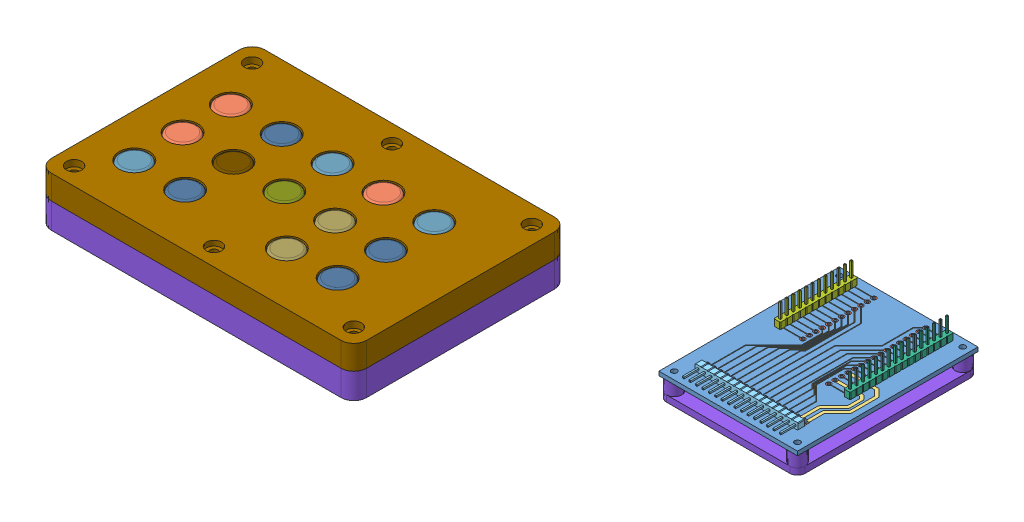
SolidWorks assembly central_station, configuration Default. Lengths in mm.
Overall size (285.1 66.66 84.42).
110 component instances, 27 part files, 11 mates.
Components (placement in the parent):
- controller1-controller.step-1: controller1-controller.step [Default] at (-1.9609 35.1675 90.037) x (1 0 0) z (0 1 0) size (54.5 71 11.54)
  - Board_Geoms_2cbe.step-1: Board_Geoms_2cbe.step [Default] at origin size (54.5 71 1.65)
    - Pcb_2cbe.step-1: Pcb_2cbe.step [Default] at (-119.5 126 0) size (54.5 71 1.6)
    - topPads_2cbe.step-1: topPads_2cbe.step [Default] at (-119.5 126 0.02) size (39.81 57.72 0.01)
    - topTracks_2cbe.step-1: topTracks_2cbe.step [Default] at (-119.5 126 0.01) size (44.1 56.73 0.01)
    - botPads_2cbe.step-1: botPads_2cbe.step [Default] at (-119.5 126 -1.62) size (39.81 57.72 0.01)
  - Step_Models_2cbe.step-1: Step_Models_2cbe.step [Default] at origin size (40.64 67.26 11.54)
    - Top_2cbe.step-1: Top_2cbe.step [Default] at origin size (40.64 67.26 11.54)
      - J3_PinHeader_1x16_P254mm_Horizontal_6185DDD9.step-1: J3_PinHeader_1x16_P254mm_Horizontal_6185DDD9.step [Default] at (46.34 11.21 0) x (0 -1 0) z (0 0 1) size (10.36 40.64 5.54)
      - J2_PinHeader_1x16_P254mm_Vertical_6185DCF0.step-1: J2_PinHeader_1x16_P254mm_Vertical_6185DCF0.step [Default] at (46.14 29.06 0) x (-1 0 0) z (0 0 1) size (2.54 40.64 11.54)
      - J1_PinHeader_1x12_P254mm_Vertical_6185DCCC.step-1: J1_PinHeader_1x12_P254mm_Vertical_6185DCCC.step [Default] at (8.52 67.16 0) size (2.54 30.48 11.54)
- base-1: base [Default] at (68.1365 26.0675 3.2619) size (54.5 7.5 71)
- Control_pad1-Control_pad.step-1: Control_pad1-Control_pad.step [Default] at (-325.562 -13.3521 -38.5409) x (1 0 0) z (0 1 0) size (120 80 13.4)
  - Board_Geoms_9430.step-1: Board_Geoms_9430.step [Default] at origin size (120 80 1.6)
    - Pcb_9430.step-1: Pcb_9430.step [Default] at origin size (120 80 1.6)
  - Step_Models_9430.step-1: Step_Models_9430.step [Default] at origin size (106.29 65.25 13.4)
    - Top_9430.step-1: Top_9430.step [Default] at origin size (106.29 65.25 13.4)
      - S2__2mmx12mm_With_White_cap_round_6188A434.step-1: S2__2mmx12mm_With_White_cap_round_6188A434.step [Default] at (130 -83.35 0) size (13.42 13 13.05)
        - round-cap.step-1: round-cap.step [Default] at origin size (13 13 7.7)
        - Tactal_Switch_-_THRU(12mmx12mmx__mm)-Square_Yellow.step-1: Tactal_Switch_-_THRU(12mmx12mmx__mm)-Square_Yellow.step [Default] at origin size (13.42 12.01 10.79)
      - S2__2mmx12mm_With_White_cap_round_6188A434.step-2: S2__2mmx12mm_With_White_cap_round_6188A434.step [Default] at (190 -121.35 0) size (13.42 13 13.05)
        - round-cap.step-1: round-cap.step [Default] at origin size (13 13 7.7)
        - Tactal_Switch_-_THRU(12mmx12mmx__mm)-Square_Yellow.step-1: Tactal_Switch_-_THRU(12mmx12mmx__mm)-Square_Yellow.step [Default] at origin size (13.42 12.01 10.79)
      - S13__2mmx12mm_With_Yellow_cap_round_inf.step-1: S13__2mmx12mm_With_Yellow_cap_round_inf.step [Default] at (170 -121.35 0) size (13.42 13 13.05)
        - round-cap001.step-1: round-cap001.step [Default] at origin size (13 13 7.7)
        - Tactal_Switch_-_THRU(12mmx12mmx__mm)-Square_Yellow001.step-1: Tactal_Switch_-_THRU(12mmx12mmx__mm)-Square_Yellow001.step [Default] at origin size (13.42 12.01 10.79)
      - S2__2mmx12mm_With_White_cap_round_6188A434.step-3: S2__2mmx12mm_With_White_cap_round_6188A434.step [Default] at (130 -121.35 0) size (13.42 13 13.05)
        - round-cap.step-1: round-cap.step [Default] at origin size (13 13 7.7)
        - Tactal_Switch_-_THRU(12mmx12mmx__mm)-Square_Yellow.step-1: Tactal_Switch_-_THRU(12mmx12mmx__mm)-Square_Yellow.step [Default] at origin size (13.42 12.01 10.79)
      - S11__2mmx12mm_With_Red_cap_round_6188A4B2.step-1: S11__2mmx12mm_With_Red_cap_round_6188A4B2.step [Default] at (110 -121.35 0) size (13.42 13 13.05)
        - round-cap002.step-1: round-cap002.step [Default] at origin size (13 13 7.7)
        - Tactal_Switch_-_THRU(12mmx12mmx__mm)-Square_Yellow002.step-1: Tactal_Switch_-_THRU(12mmx12mmx__mm)-Square_Yellow002.step [Default] at origin size (13.42 12.01 10.79)
      - S2__2mmx12mm_With_White_cap_round_6188A434.step-4: S2__2mmx12mm_With_White_cap_round_6188A434.step [Default] at (190 -102.35 0) size (13.42 13 13.05)
        - round-cap.step-1: round-cap.step [Default] at origin size (13 13 7.7)
        - Tactal_Switch_-_THRU(12mmx12mmx__mm)-Square_Yellow.step-1: Tactal_Switch_-_THRU(12mmx12mmx__mm)-Square_Yellow.step [Default] at origin size (13.42 12.01 10.79)
      - S13__2mmx12mm_With_Yellow_cap_round_inf.step-2: S13__2mmx12mm_With_Yellow_cap_round_inf.step [Default] at (170 -102.35 0) size (13.42 13 13.05)
        - round-cap001.step-1: round-cap001.step [Default] at origin size (13 13 7.7)
        - Tactal_Switch_-_THRU(12mmx12mmx__mm)-Square_Yellow001.step-1: Tactal_Switch_-_THRU(12mmx12mmx__mm)-Square_Yellow001.step [Default] at origin size (13.42 12.01 10.79)
      - S8__2mmx12mm_With_Black_cap_round_6188A488.step-1: S8__2mmx12mm_With_Black_cap_round_6188A488.step [Default] at (150 -102.35 0) size (13.42 13 13.05)
        - round-cap003.step-1: round-cap003.step [Default] at origin size (13 13 7.7)
        - Tactal_Switch_-_THRU(12mmx12mmx__mm)-Square_Yellow003.step-1: Tactal_Switch_-_THRU(12mmx12mmx__mm)-Square_Yellow003.step [Default] at origin size (13.42 12.01 10.79)
      - S7__2mmx12mm_With_Blue_cap_round_6188A47A.step-1: S7__2mmx12mm_With_Blue_cap_round_6188A47A.step [Default] at (130 -102.35 0) size (13.42 13 13.05)
        - round-cap004.step-1: round-cap004.step [Default] at origin size (13 13 7.7)
        - Tactal_Switch_-_THRU(12mmx12mmx__mm)-Square_Yellow004.step-1: Tactal_Switch_-_THRU(12mmx12mmx__mm)-Square_Yellow004.step [Default] at origin size (13.42 12.01 10.79)
      - S6__2mmx12mm_With_Green_cap_round_6188A46C.step-1: S6__2mmx12mm_With_Green_cap_round_6188A46C.step [Default] at (110 -102.35 0) size (13.42 13 13.05)
        - round-cap005.step-1: round-cap005.step [Default] at origin size (13 13 7.7)
        - Tactal_Switch_-_THRU(12mmx12mmx__mm)-Square_Yellow005.step-1: Tactal_Switch_-_THRU(12mmx12mmx__mm)-Square_Yellow005.step [Default] at origin size (13.42 12.01 10.79)
      - S11__2mmx12mm_With_Red_cap_round_6188A4B2.step-2: S11__2mmx12mm_With_Red_cap_round_6188A4B2.step [Default] at (190 -83.35 0) size (13.42 13 13.05)
        - round-cap002.step-1: round-cap002.step [Default] at origin size (13 13 7.7)
        - Tactal_Switch_-_THRU(12mmx12mmx__mm)-Square_Yellow002.step-1: Tactal_Switch_-_THRU(12mmx12mmx__mm)-Square_Yellow002.step [Default] at origin size (13.42 12.01 10.79)
      - S6__2mmx12mm_With_Green_cap_round_6188A46C.step-2: S6__2mmx12mm_With_Green_cap_round_6188A46C.step [Default] at (170 -83.35 0) size (13.42 13 13.05)
        - round-cap005.step-1: round-cap005.step [Default] at origin size (13 13 7.7)
        - Tactal_Switch_-_THRU(12mmx12mmx__mm)-Square_Yellow005.step-1: Tactal_Switch_-_THRU(12mmx12mmx__mm)-Square_Yellow005.step [Default] at origin size (13.42 12.01 10.79)
      - S11__2mmx12mm_With_Red_cap_round_6188A4B2.step-3: S11__2mmx12mm_With_Red_cap_round_6188A4B2.step [Default] at (150 -83.35 0) size (13.42 13 13.05)
        - round-cap002.step-1: round-cap002.step [Default] at origin size (13 13 7.7)
        - Tactal_Switch_-_THRU(12mmx12mmx__mm)-Square_Yellow002.step-1: Tactal_Switch_-_THRU(12mmx12mmx__mm)-Square_Yellow002.step [Default] at origin size (13.42 12.01 10.79)
      - S6__2mmx12mm_With_Green_cap_round_6188A46C.step-3: S6__2mmx12mm_With_Green_cap_round_6188A46C.step [Default] at (110 -83.35 0) size (13.42 13 13.05)
        - round-cap005.step-1: round-cap005.step [Default] at origin size (13 13 7.7)
        - Tactal_Switch_-_THRU(12mmx12mmx__mm)-Square_Yellow005.step-1: Tactal_Switch_-_THRU(12mmx12mmx__mm)-Square_Yellow005.step [Default] at origin size (13.42 12.01 10.79)
      - R29_R_0805_2012Metric_6188A418.step-1: R29_R_0805_2012Metric_6188A418.step [Default] at (193.33 -112.45 0) x (0 -1 0) z (0 0 1) size (2 1.2 0.45)
      - R29_R_0805_2012Metric_6188A418.step-2: R29_R_0805_2012Metric_6188A418.step [Default] at (173.3 -112.45 0) x (0 -1 0) z (0 0 1) size (2 1.2 0.45)
      - R29_R_0805_2012Metric_6188A418.step-3: R29_R_0805_2012Metric_6188A418.step [Default] at (133.24 -112.45 0) x (0 -1 0) z (0 0 1) size (2 1.2 0.45)
      - R29_R_0805_2012Metric_6188A418.step-4: R29_R_0805_2012Metric_6188A418.step [Default] at (113.21 -112.45 0) x (0 -1 0) z (0 0 1) size (2 1.2 0.45)
      - R29_R_0805_2012Metric_6188A418.step-5: R29_R_0805_2012Metric_6188A418.step [Default] at (193.33 -93.48 0) x (0 -1 0) z (0 0 1) size (2 1.2 0.45)
      - R29_R_0805_2012Metric_6188A418.step-6: R29_R_0805_2012Metric_6188A418.step [Default] at (173.3 -93.48 0) x (0 -1 0) z (0 0 1) size (2 1.2 0.45)
      - R29_R_0805_2012Metric_6188A418.step-7: R29_R_0805_2012Metric_6188A418.step [Default] at (153.27 -93.48 0) x (0 -1 0) z (0 0 1) size (2 1.2 0.45)
      - R29_R_0805_2012Metric_6188A418.step-8: R29_R_0805_2012Metric_6188A418.step [Default] at (208 -94.44 0) x (-1 0 0) z (0 0 1) size (2 1.2 0.45)
      - R29_R_0805_2012Metric_6188A418.step-9: R29_R_0805_2012Metric_6188A418.step [Default] at (133.24 -93.48 0) x (0 -1 0) z (0 0 1) size (2 1.2 0.45)
      - R29_R_0805_2012Metric_6188A418.step-10: R29_R_0805_2012Metric_6188A418.step [Default] at (113.21 -93.48 0) x (0 -1 0) z (0 0 1) size (2 1.2 0.45)
      - R29_R_0805_2012Metric_6188A418.step-11: R29_R_0805_2012Metric_6188A418.step [Default] at (193.33 -73.92 0) x (0 -1 0) z (0 0 1) size (2 1.2 0.45)
      - R29_R_0805_2012Metric_6188A418.step-12: R29_R_0805_2012Metric_6188A418.step [Default] at (173.27 -73.98 0) x (0 -1 0) z (0 0 1) size (2 1.2 0.45)
      - R29_R_0805_2012Metric_6188A418.step-13: R29_R_0805_2012Metric_6188A418.step [Default] at (153.26 -73.95 0) x (0 -1 0) z (0 0 1) size (2 1.2 0.45)
      - R29_R_0805_2012Metric_6188A418.step-14: R29_R_0805_2012Metric_6188A418.step [Default] at (133.27 -73.98 0) x (0 -1 0) z (0 0 1) size (2 1.2 0.45)
      - R29_R_0805_2012Metric_6188A418.step-15: R29_R_0805_2012Metric_6188A418.step [Default] at (113.22 -73.96 0) x (0 -1 0) z (0 0 1) size (2 1.2 0.45)
      - J4_JST_B4B_XH_A_6188A22B.step-1: J4_JST_B4B_XH_A_6188A22B.step [Default] at (197 -66 0) x (-1 0 0) z (0 0 1) size (12.4 5.75 10.4)
      - J4_JST_B4B_XH_A_6188A22B.step-2: J4_JST_B4B_XH_A_6188A22B.step [Default] at (182 -66 0) x (-1 0 0) z (0 0 1) size (12.4 5.75 10.4)
      - J4_JST_B4B_XH_A_6188A22B.step-3: J4_JST_B4B_XH_A_6188A22B.step [Default] at (135 -66 0) x (-1 0 0) z (0 0 1) size (12.4 5.75 10.4)
      - J4_JST_B4B_XH_A_6188A22B.step-4: J4_JST_B4B_XH_A_6188A22B.step [Default] at (120 -66 0) x (-1 0 0) z (0 0 1) size (12.4 5.75 10.4)
      - D1_LED_1206_3216Metric_6188A17F.step-1: D1_LED_1206_3216Metric_6188A17F.step [Default] at (207.9775 -97.02 0) x (-1 0 0) z (0 0 1) size (3.2 1.6 1.1)
      - C14_C_0805_2012Metric_6188A16C.step-1: C14_C_0805_2012Metric_6188A16C.step [Default] at (195.4 -112.42 0) x (0 -1 0) z (0 0 1) size (2 1.25 1.25)
      - C14_C_0805_2012Metric_6188A16C.step-2: C14_C_0805_2012Metric_6188A16C.step [Default] at (175.39 -112.42 0) x (0 -1 0) z (0 0 1) size (2 1.25 1.25)
      - C14_C_0805_2012Metric_6188A16C.step-3: C14_C_0805_2012Metric_6188A16C.step [Default] at (135.37 -112.42 0) x (0 -1 0) z (0 0 1) size (2 1.25 1.25)
      - C14_C_0805_2012Metric_6188A16C.step-4: C14_C_0805_2012Metric_6188A16C.step [Default] at (115.36 -112.45 0) x (0 -1 0) z (0 0 1) size (2 1.25 1.25)
      - C14_C_0805_2012Metric_6188A16C.step-5: C14_C_0805_2012Metric_6188A16C.step [Default] at (195.4 -93.48 0) x (0 -1 0) z (0 0 1) size (2 1.25 1.25)
      - C14_C_0805_2012Metric_6188A16C.step-6: C14_C_0805_2012Metric_6188A16C.step [Default] at (175.39 -93.48 0) x (0 -1 0) z (0 0 1) size (2 1.25 1.25)
      - C14_C_0805_2012Metric_6188A16C.step-7: C14_C_0805_2012Metric_6188A16C.step [Default] at (155.38 -93.48 0) x (0 -1 0) z (0 0 1) size (2 1.25 1.25)
      - C14_C_0805_2012Metric_6188A16C.step-8: C14_C_0805_2012Metric_6188A16C.step [Default] at (135.37 -93.48 0) x (0 -1 0) z (0 0 1) size (2 1.25 1.25)
      - C14_C_0805_2012Metric_6188A16C.step-9: C14_C_0805_2012Metric_6188A16C.step [Default] at (115.36 -93.48 0) x (0 -1 0) z (0 0 1) size (2 1.25 1.25)
      - C14_C_0805_2012Metric_6188A16C.step-10: C14_C_0805_2012Metric_6188A16C.step [Default] at (195.4 -73.99 0) x (0 -1 0) z (0 0 1) size (2 1.25 1.25)
      - C14_C_0805_2012Metric_6188A16C.step-11: C14_C_0805_2012Metric_6188A16C.step [Default] at (175.3925 -73.99 0) x (0 -1 0) z (0 0 1) size (2 1.25 1.25)
      - C14_C_0805_2012Metric_6188A16C.step-12: C14_C_0805_2012Metric_6188A16C.step [Default] at (155.385 -73.99 0) x (0 -1 0) z (0 0 1) size (2 1.25 1.25)
      - C14_C_0805_2012Metric_6188A16C.step-13: C14_C_0805_2012Metric_6188A16C.step [Default] at (135.3775 -73.99 0) x (0 -1 0) z (0 0 1) size (2 1.25 1.25)
      - C14_C_0805_2012Metric_6188A16C.step-14: C14_C_0805_2012Metric_6188A16C.step [Default] at (115.37 -73.99 0) x (0 -1 0) z (0 0 1) size (2 1.25 1.25)
    - Bot_9430.step-1: Bot_9430.step [Default] at origin size (82.77 39.2 0.45)
      - R29_R_0805_2012Metric_6188A418.step-1: R29_R_0805_2012Metric_6188A418.step [Default] at (191.94 -118.81 -1.6) x (-1 0 0) z (0 0 -1) size (2 1.2 0.45)
      - R29_R_0805_2012Metric_6188A418.step-2: R29_R_0805_2012Metric_6188A418.step [Default] at (171.77 -118.81 -1.6) x (-1 0 0) z (0 0 -1) size (2 1.2 0.45)
      - R29_R_0805_2012Metric_6188A418.step-3: R29_R_0805_2012Metric_6188A418.step [Default] at (131.39 -118.81 -1.6) x (-1 0 0) z (0 0 -1) size (2 1.2 0.45)
      - R29_R_0805_2012Metric_6188A418.step-4: R29_R_0805_2012Metric_6188A418.step [Default] at (111.2 -118.81 -1.6) x (-1 0 0) z (0 0 -1) size (2 1.2 0.45)
      - R29_R_0805_2012Metric_6188A418.step-5: R29_R_0805_2012Metric_6188A418.step [Default] at (191.96 -99.81 -1.6) x (-1 0 0) z (0 0 -1) size (2 1.2 0.45)
      - R29_R_0805_2012Metric_6188A418.step-6: R29_R_0805_2012Metric_6188A418.step [Default] at (171.77 -99.81 -1.6) x (-1 0 0) z (0 0 -1) size (2 1.2 0.45)
      - R29_R_0805_2012Metric_6188A418.step-7: R29_R_0805_2012Metric_6188A418.step [Default] at (151.58 -99.81 -1.6) x (-1 0 0) z (0 0 -1) size (2 1.2 0.45)
      - R29_R_0805_2012Metric_6188A418.step-8: R29_R_0805_2012Metric_6188A418.step [Default] at (131.39 -99.81 -1.6) x (-1 0 0) z (0 0 -1) size (2 1.2 0.45)
      - R29_R_0805_2012Metric_6188A418.step-9: R29_R_0805_2012Metric_6188A418.step [Default] at (111.19 -99.81 -1.6) x (-1 0 0) z (0 0 -1) size (2 1.2 0.45)
      - R29_R_0805_2012Metric_6188A418.step-10: R29_R_0805_2012Metric_6188A418.step [Default] at (191.96 -80.81 -1.6) x (-1 0 0) z (0 0 -1) size (2 1.2 0.45)
      - R29_R_0805_2012Metric_6188A418.step-11: R29_R_0805_2012Metric_6188A418.step [Default] at (171.77 -80.81 -1.6) x (-1 0 0) z (0 0 -1) size (2 1.2 0.45)
      - R29_R_0805_2012Metric_6188A418.step-12: R29_R_0805_2012Metric_6188A418.step [Default] at (151.58 -80.81 -1.6) x (-1 0 0) z (0 0 -1) size (2 1.2 0.45)
      - R29_R_0805_2012Metric_6188A418.step-13: R29_R_0805_2012Metric_6188A418.step [Default] at (131.39 -80.81 -1.6) x (-1 0 0) z (0 0 -1) size (2 1.2 0.45)
      - R29_R_0805_2012Metric_6188A418.step-14: R29_R_0805_2012Metric_6188A418.step [Default] at (111.2 -80.81 -1.6) x (-1 0 0) z (0 0 -1) size (2 1.2 0.45)
- pad_base-1: pad_base [Default] at (-11.249 -22.9521 17.5187) size (124 10 84)
- pad_lid-1: pad_lid [Default] at (250.3236 -12.9521 -12.6381) size (124 9.5 84)
Mates (geometry in assembly coordinates):
- Concentric1: concentric aligned: cylinder of controller1-controller.step-1/Board_Geoms_2cbe.step-1/Pcb_2cbe.step-1 through (49.5391 35.1675 87.037) axis (0 1 0) radius 1.1; cylinder of base-1 through (49.5391 21.8249 87.037) axis (0 1 0) radius 1.5
- Distance1: distance = 2 mm aligned: plane of pad_base-1 through (-232.562 -12.9521 103.4591) normal (0 0 1); plane of Control_pad1-Control_pad.step-1/Board_Geoms_9430.step-1/Pcb_9430.step-1 through (-225.562 -13.3521 101.4591) normal (0 0 1)
- Distance2: distance = 2 mm aligned: plane of pad_base-1 through (-232.562 -12.9521 19.4591) normal (-1 0 0); plane of Control_pad1-Control_pad.step-1/Board_Geoms_9430.step-1/Pcb_9430.step-1 through (-230.562 -13.3521 26.4591) normal (-1 0 0)
- Parallel1: parallel anti-aligned: plane of Control_pad1-Control_pad.step-1/Board_Geoms_9430.step-1/Pcb_9430.step-1 through (-170.562 -14.9521 61.4591) normal (0 -1 0); plane of pad_base-1 through (-11.249 -14.9521 17.5187) normal (0 1 0)
- Coincident6: coincident anti-aligned: plane of Control_pad1-Control_pad.step-1/Board_Geoms_9430.step-1/Pcb_9430.step-1 through (-170.562 -14.9521 61.4591) normal (0 -1 0); plane of pad_base-1 through (-11.249 -14.9521 17.5187) normal (0 1 0)
- Coincident7: coincident anti-aligned: plane of Control_pad1-Control_pad.step-1/Board_Geoms_9430.step-1/Pcb_9430.step-1 through (-170.562 -14.9521 61.4591) normal (0 -1 0); plane of pad_base-1 through (-11.249 -14.9521 17.5187) normal (0 1 0)
- Coincident8: coincident anti-aligned: plane of Control_pad1-Control_pad.step-1/Board_Geoms_9430.step-1/Pcb_9430.step-1 through (-170.562 -14.9521 61.4591) normal (0 -1 0); plane of pad_base-1 through (-11.249 -14.9521 17.5187) normal (0 1 0)
- Coincident9: coincident anti-aligned: plane of pad_base-1 through (-11.249 -12.9521 17.5187) normal (0 1 0); plane of pad_lid-1 through (250.3236 -12.9521 -12.6381) normal (0 -1 0)
- Coincident10: coincident aligned: plane of pad_base-1 through (-232.562 -12.9521 19.4591) normal (-1 0 0); plane of pad_lid-1 through (-232.562 -3.4521 19.4591) normal (-1 0 0)
- Coincident11: coincident aligned: plane of pad_base-1 through (-232.562 -12.9521 103.4591) normal (0 0 1); plane of pad_lid-1 through (-232.562 -3.4521 103.4591) normal (0 0 1)
- Coincident12: coincident anti-aligned: plane of pad_base-1 through (-11.249 -12.9521 17.5187) normal (0 1 0); plane of pad_lid-1 through (250.3236 -12.9521 -12.6381) normal (0 -1 0)
